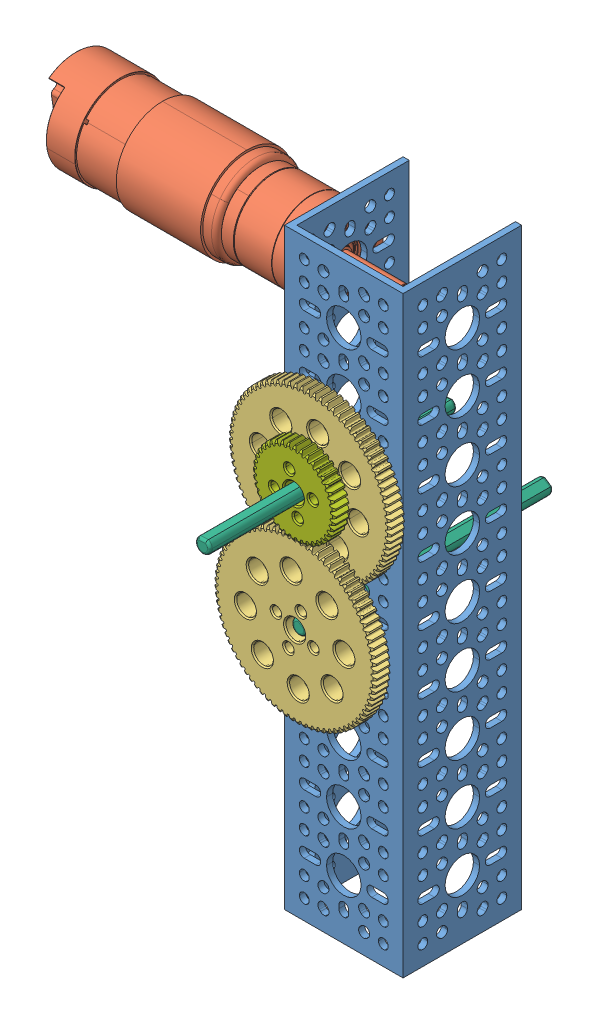
SolidWorks assembly Ball Launcher, configuration Default. Lengths in mm.
Overall size (174.14 240 138.98).
11 component instances, 7 part files, 21 mates.
Components (placement in the parent):
- 1120-0009-0240.step-1: 1120-0009-0240.step [Default] at (-49.2711 21.1308 268.2009) size (48 240 48)
- 5202-0002-0005 part.step-1: 5202-0002-0005 part.step [Default] at (-181.7711 237.1308 246.7009) x (0 0.98793 0.154902) z (-1 0 0) size (37.5 37.5 132.7)
- 39086_txm-gear80-tooth.step-1: 39086_txm-gear80-tooth.step [Default] at (-74.7566 190.6526 244.0115) x (0 0 -1) z (0.976544 0.21532 0) size (6.37 65.59 65.59)
- 39079_txm-motor shaft hub with set screw.step-1: 39079_txm-motor shaft hub with set screw.step [Default] at (-48.4472 172.174 260.2532) x (0.976544 0.21532 0) z (0 0 1) size (22 22 9.4)
- 1611-0514-0006.step-2: 1611-0514-0006.step [Default] at (-49.2711 189.1308 266.7009) x (0.573511 -0.819198 0) z (-0.819198 -0.573511 0) size (15 5 15)
- 44708_txp-6mm x 100mmaxle.step-1: 44708_txp-6mm x 100mmaxle.step [Default] at (-88.0698 144.3324 212.7991) x (0.997363 0.072577 0) z (0 0 1) size (6 5.5 100)
- 39028_txm-gear40-tooth.step-2: 39028_txm-gear40-tooth.step [Default] at (-56.7838 185.4492 269.9744) x (0 0 -1) z (0.976544 0.21532 0) size (6.36 33.59 33.59)
- 1611-0514-0006.step-3: 1611-0514-0006.step [Default] at (-49.2711 141.1308 266.7009) x (0.943683 0.33085 0) z (0.33085 -0.943683 0) size (15 5 15)
- 44708_txp-6mm x 100mmaxle.step-2: 44708_txp-6mm x 100mmaxle.step [Default] at (-107.3757 129.465 173.8194) x (0.833013 -0.553254 0) z (0 0 1) size (6 5.5 100)
- 39086_txm-gear80-tooth.step-2: 39086_txm-gear80-tooth.step [Default] at (-70.3946 155.4705 249.8615) x (0 0 -1) z (0.949321 -0.314309 0) size (6.37 65.59 65.59)
- 39079_txm-motor shaft hub with set screw.step-3: 39079_txm-motor shaft hub with set screw.step [Default] at (-57.2338 126.1372 266.1032) x (0.949321 -0.314309 0) z (0 0 1) size (22 22 9.4)
Mates (geometry in assembly coordinates):
- Concentric7: concentric: cylinder of 39086_txm-gear80-tooth.step-1 through (-49.2711 189.1308 231.5757) axis (0 0 1) radius 4; cylinder of 39079_txm-motor shaft hub with set screw.step-1 through (-49.2711 189.1308 281.1009) axis (0 0 -1) radius 3.9625
- Concentric8: concentric: cylinder of 39086_txm-gear80-tooth.step-1 through (-47.5486 181.3184 289.9834) axis (0 0 -1) radius 1.85; circle of 39079_txm-motor shaft hub with set screw.step-1
- Coincident8: coincident: plane of 39086_txm-gear80-tooth.step-1 through (-49.2711 189.1308 278.4009) normal (0 0 -1); plane of 39079_txm-motor shaft hub with set screw.step-1 through (-49.2711 189.1308 278.4009) normal (0 0 1)
- Concentric12: concentric: cylinder of 1120-0009-0240.step-1 through (-49.2711 189.1308 260.7009) axis (0 0 1) radius 7; cylinder of 1611-0514-0006.step-2 through (-49.2711 189.1308 270.7009) axis (0 0 -1) radius 7
- Coincident10: coincident: plane of 1120-0009-0240.step-1 through (-25.2711 261.1308 270.7009) normal (0 0 1); plane of 1611-0514-0006.step-2 through (-49.2711 189.1308 270.7009) normal (0 0 -1)
- Concentric13: concentric: cylinder of 1611-0514-0006.step-2 through (-49.2711 189.1308 266.7009) axis (0 0 1) radius 3; cylinder of 44708_txp-6mm x 100mmaxle.step-1 through (-49.2711 189.1308 327.9195) axis (0 0 -1) radius 3
- Concentric14: concentric: cylinder of 39079_txm-motor shaft hub with set screw.step-1 through (-49.2711 189.1308 271.7009) axis (0 0 1) radius 3.015; cylinder of 44708_txp-6mm x 100mmaxle.step-1 through (-49.2711 189.1308 327.9195) axis (0 0 -1) radius 3
- Coincident11: coincident: plane of 39079_txm-motor shaft hub with set screw.step-1 through (-49.2711 189.1308 271.7009) normal (0 0 -1); plane of 1611-0514-0006.step-2 through (-49.2711 189.1308 271.7009) normal (0 0 1)
- Concentric15: concentric: cylinder of 44708_txp-6mm x 100mmaxle.step-1 through (-49.2711 189.1308 327.9195) axis (0 0 -1) radius 3; cylinder of 39028_txm-gear40-tooth.step-2 through (-49.2711 189.1308 237.9258) axis (0 0 1) radius 4
- Concentric16: concentric: cylinder of 39086_txm-gear80-tooth.step-1 through (-50.9937 196.9431 289.9834) axis (0 0 -1) radius 1.85; cylinder of 39028_txm-gear40-tooth.step-2 through (-50.9937 196.9431 291.1009) axis (0 0 -1) radius 1.85
- Coincident13: coincident: plane of 39086_txm-gear80-tooth.step-1 through (-49.2711 189.1308 284.7509) normal (0 0 1); plane of 39028_txm-gear40-tooth.step-2 through (-49.2711 189.1308 284.7509) normal (0 0 -1)
- Concentric17: concentric: cylinder of 1120-0009-0240.step-1 through (-49.2711 141.1308 260.7009) axis (0 0 1) radius 7; cylinder of 1611-0514-0006.step-3 through (-49.2711 141.1308 270.7009) axis (0 0 -1) radius 7
- Coincident14: coincident: plane of 1120-0009-0240.step-1 through (-25.2711 261.1308 270.7009) normal (0 0 1); plane of 1611-0514-0006.step-3 through (-49.2711 141.1308 270.7009) normal (0 0 -1)
- Concentric18: concentric: cylinder of 1611-0514-0006.step-3 through (-49.2711 141.1308 266.7009) axis (0 0 1) radius 3; cylinder of 44708_txp-6mm x 100mmaxle.step-2 through (-49.2711 141.1308 288.9398) axis (0 0 -1) radius 3
- Concentric19: concentric: cylinder of 44708_txp-6mm x 100mmaxle.step-2 through (-49.2711 141.1308 288.9398) axis (0 0 -1) radius 3; cylinder of 39086_txm-gear80-tooth.step-2 through (-49.2711 141.1308 237.4257) axis (0 0 1) radius 4
- Coincident15: coincident: circle of 39086_txm-gear80-tooth.step-1; plane of 39086_txm-gear80-tooth.step-2 through (-49.2711 141.1308 284.2509) normal (0 0 -1)
- Concentric20: concentric: cylinder of 44708_txp-6mm x 100mmaxle.step-2 through (-49.2711 141.1308 288.9398) axis (0 0 -1) radius 3; cylinder of 39079_txm-motor shaft hub with set screw.step-3 through (-49.2711 141.1308 277.5509) axis (0 0 1) radius 3.015
- Coincident16: coincident: plane of 39086_txm-gear80-tooth.step-2 through (-49.2711 141.1308 284.2509) normal (0 0 -1); plane of 39079_txm-motor shaft hub with set screw.step-3 through (-49.2711 141.1308 284.2509) normal (0 0 1)
- Concentric21: concentric: cylinder of 39086_txm-gear80-tooth.step-2 through (-46.7567 148.7253 295.8334) axis (0 0 -1) radius 1.85; circle of 39079_txm-motor shaft hub with set screw.step-3
- Coincident20: coincident: circle of 1120-0009-0240.step-1; circle of 5202-0002-0005 part.step-1
- Concentric29: concentric: cylinder of 1120-0009-0240.step-1 through (-63.2711 237.1308 246.7009) axis (-1 0 0) radius 7; cylinder of 5202-0002-0005 part.step-1 through (-49.2711 237.1308 246.7009) axis (-1 0 0) radius 3
